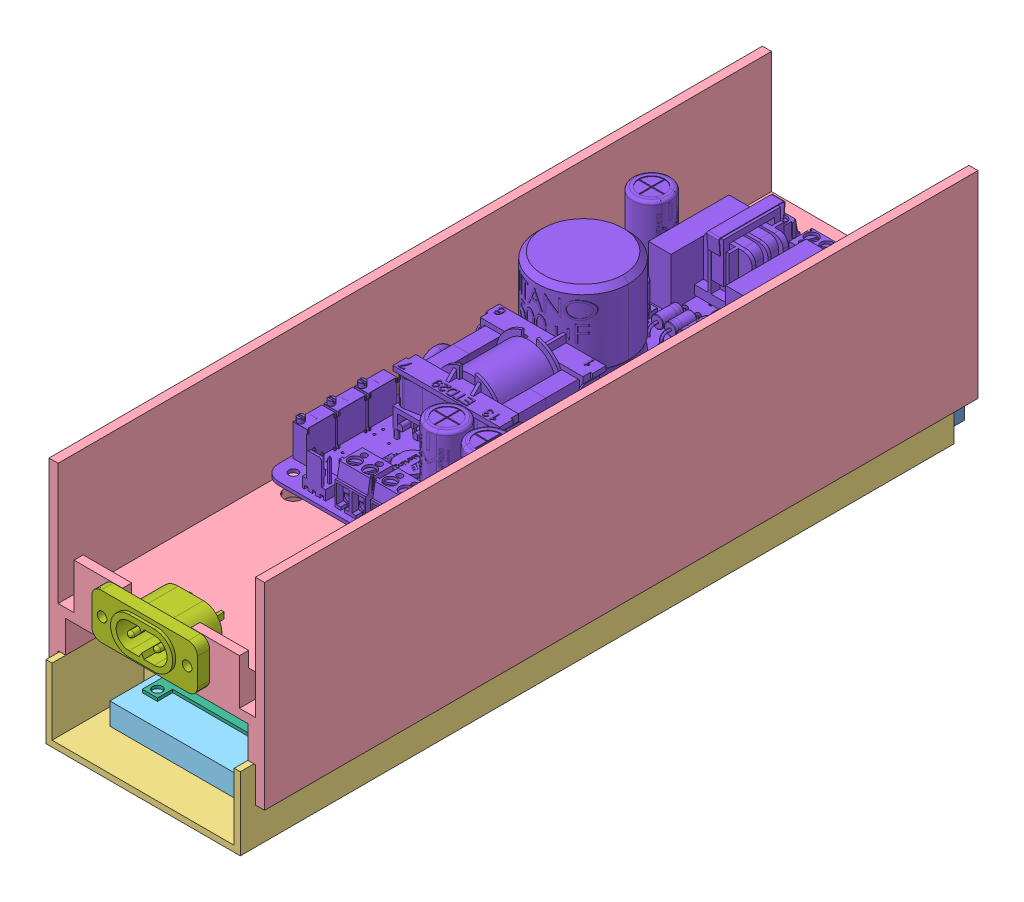
SolidWorks assembly АКБ AED, сборка, configuration Default. Lengths in mm.
Overall size (71 77.5 242).
8 component instances, 8 part files, 23 mates.
Components (placement in the parent):
- Корпус платы АКБ AED-1: Корпус платы АКБ AED [Default] at origin size (58 32 195)
- Плата БП AED-1: Плата БП AED [Default] at (0 -2.45 13.625) size (51 1.3 48.75)
- АКБ AED, корпус программатора-1: АКБ AED, корпус программатора [Default] at (0 1 51.4854) size (64 24 235)
- АКБ AED, корпус БП-1: АКБ AED, корпус БП [Default] at origin size (71 65 235)
- АКБ AED, держатель платы программатора-1: АКБ AED, держатель платы программатора [Default] at (0 1 51.4854) size (59.5 20 22.95)
- АКБ AED, плата программатора-1: АКБ AED, плата программатора [Default] at (0 -0.8 38.8067) x (-1 0 0) z (0 -1 0) size (43 34 1)
- KLS1-AS-222-12-1: KLS1-AS-222-12 [Default] at (0 33.95 84) size (34.8 14.9 21.5)
- POWER_SUPPLY_20V_4A.step-2: POWER_SUPPLY_20V_4A.step [Default] at (-30 32.5914 -133) x (0 0 1) z (0 1 0) size (150 60.42 51.54)
Mates (geometry in assembly coordinates):
- Width1: width aligned: plane of Корпус платы АКБ AED-1 through (-29 9 40) normal (-1 0 0); plane of Плата БП AED-1 through (29 9 40) normal (1 0 0); plane of Корпус платы АКБ AED-1 through (-23.25 -1.8 35.2) normal (-1 0 0); plane of Плата БП AED-1 through (23.25 -1.8 22.5) normal (1 0 0)
- Coincident1: coincident aligned: plane of Корпус платы АКБ AED-1 through (0 0 0) normal (0 0 1)
- Coincident2: coincident aligned: plane of Корпус платы АКБ AED-1 through (0 0 0) normal (0 1 0)
- Coincident3: coincident aligned: plane of Корпус платы АКБ AED-1 through (0 0 0) normal (1 0 0)
- Coincident5: coincident aligned: plane of Корпус платы АКБ AED-1 through (1.25 -1.8 40) normal (0 1 0); plane of Плата БП AED-1 through (24 -1.8 2.45) normal (0 1 0)
- Coincident7: coincident anti-aligned: plane of Корпус платы АКБ AED-1 through (0 0 38) normal (0 0 -1); plane of Плата БП AED-1 through (1.75 -1.8 38) normal (0 0 1)
- Width3: width aligned: plane of АКБ AED, корпус программатора-1 through (-32 -11 86.4854) normal (-1 0 0); plane of Корпус платы АКБ AED-1 through (32 -11 86.4854) normal (1 0 0); plane of АКБ AED, корпус программатора-1 through (-29 9 40) normal (-1 0 0); plane of Корпус платы АКБ AED-1 through (29 9 40) normal (1 0 0)
- Coincident8: coincident anti-aligned: plane of Корпус платы АКБ AED-1 through (-29 -9 40) normal (0 -1 0); plane of АКБ AED, корпус программатора-1 through (30 -9 86.4854) normal (0 1 0)
- InPlace1: in place: plane of ? through (0 0 0) normal (0 0 1); moOrthogonalPlaneRef_w of ? through (0 0 0) normal (0 1 0); plane of ? through (0 0 0) normal (1 0 0); unknown of ?
- Coincident9: coincident aligned: plane of assembly through (0 0 0) normal (0 0 1)
- Coincident10: coincident aligned: plane of АКБ AED, корпус БП-1 through (0 0 0) normal (0 1 0)
- Coincident11: coincident anti-aligned: plane of АКБ AED, корпус БП-1 through (0 0 0) normal (1 0 0)
- Width4: width anti-aligned: plane of АКБ AED, корпус программатора-1 through (-30 13 86.4854) normal (1 0 0); plane of АКБ AED, корпус программатора-1 through (30 -9 86.4854) normal (-1 0 0); plane of АКБ AED, держатель платы программатора-1 through (-29.75 11 52.9604) normal (-1 0 0); plane of АКБ AED, держатель платы программатора-1 through (29.75 11 52.9604) normal (1 0 0)
- Width5: width anti-aligned: plane of АКБ AED, корпус программатора-1 through (30 12 53.2354) normal (0 0 -1); plane of АКБ AED, корпус программатора-1 through (30 12 49.7354) normal (0 0 1); plane of АКБ AED, держатель платы программатора-1 through (0 1 52.9604) normal (0 0 1); plane of АКБ AED, держатель платы программатора-1 through (0 1 50.0104) normal (0 0 -1)
- Coincident11: coincident anti-aligned: plane of АКБ AED, корпус программатора-1 through (30 -9 86.4854) normal (0 1 0); plane of АКБ AED, держатель платы программатора-1 through (-29.75 -9 52.9604) normal (0 -1 0)
- Coincident15: coincident anti-aligned: plane of АКБ AED, плата программатора-1 through (0 -0.8 38.8067) normal (-1 0 0)
- Coincident17: coincident anti-aligned: plane of АКБ AED, держатель платы программатора-1 through (-23 -1.8 52.9604) normal (0 1 0); plane of АКБ AED, плата программатора-1 through (0 -1.8 38.8067) normal (0 -1 0)
- Coincident19: coincident anti-aligned: plane of АКБ AED, корпус БП-1 through (-32.5 26.5 82) normal (0 1 0); plane of KLS1-AS-222-12-1 through (-14.4 26.5 86) normal (0 -1 0)
- Coincident20: coincident aligned: plane of KLS1-AS-222-12-1 through (0 33.95 84) normal (1 0 0)
- Width6: width: plane of POWER_SUPPLY_20V_4A.step-2 through (-30 88.81 -128) normal (-1 0 0); plane of POWER_SUPPLY_20V_4A.step-2 through (30 88.81 12) normal (1 0 0); plane of АКБ AED, корпус БП-1 through (32.5 66.5 82) normal (-1 0 0); plane of АКБ AED, корпус БП-1 through (-32.5 66.5 82) normal (1 0 0)
- Coincident22: coincident anti-aligned: plane of АКБ AED, корпус БП-1 through (0 0 82) normal (0 0 1); plane of KLS1-AS-222-12-1 through (14.4 38.4 82) normal (0 0 -1)
- Concentric1: concentric: cylinder of АКБ AED, корпус БП-1 through (-25 16.5 12) axis (0 1 0) radius 3; cylinder of POWER_SUPPLY_20V_4A.step-2 through (-25 88.81 12) axis (0 -1 0) radius 1.5
- Distance1: distance = 5 mm anti-aligned: plane of POWER_SUPPLY_20V_4A.step-2 through (-25 31.5 -133) normal (0 -1 0); plane of АКБ AED, корпус БП-1 through (-32.5 26.5 82) normal (0 1 0)
